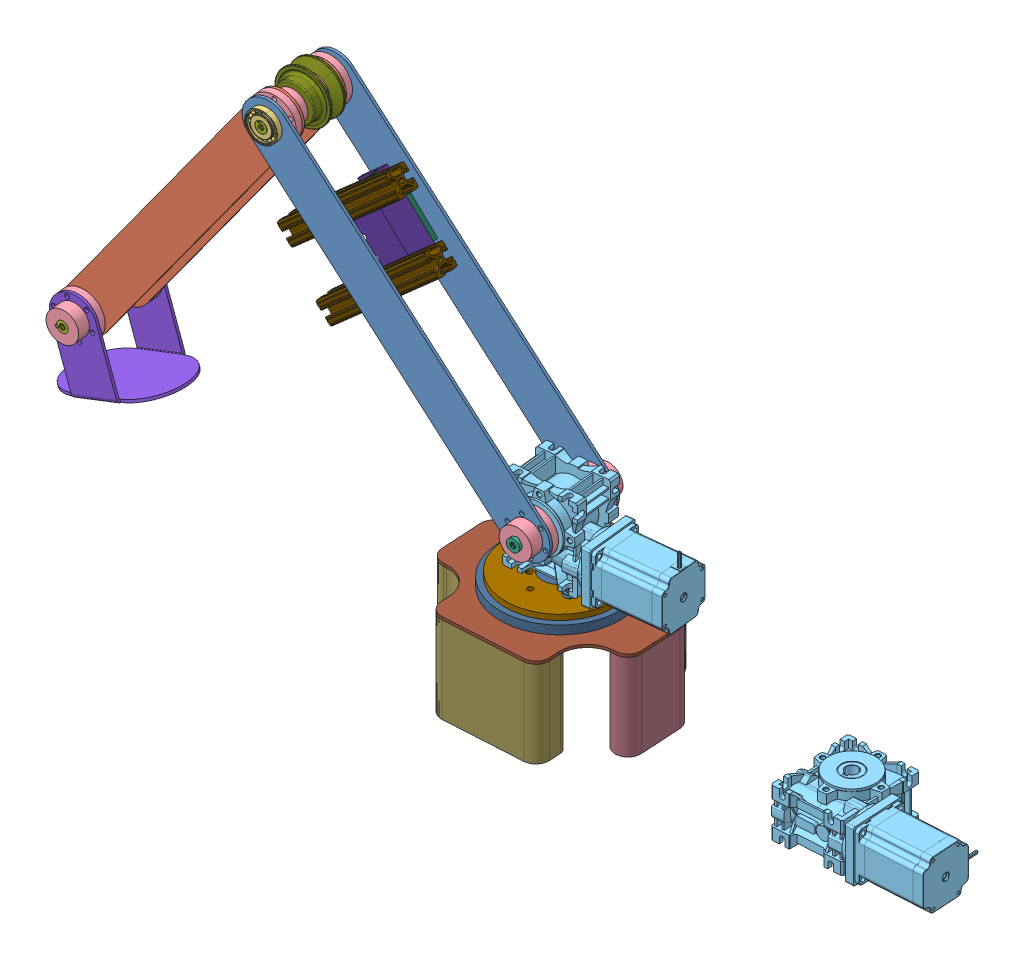
SolidWorks assembly Arm Assembly2, configuration Default. Lengths in mm.
Overall size (1007.94 520.17 219.18).
36 component instances, 19 part files, 85 mates.
Components (placement in the parent):
- Link 2-1: Link 2 [Default] at (47.0194 341.9058 298.1991) x (-0.680313 0.729219 0.073577) z (0.107525 0 0.994202) size (457.2 50.8 3.17)
- Link 3-1: Link 3 [Default] at (-260.6998 635.5723 404.1998) x (-0.575088 -0.815724 0.062197) z (0.107525 0 0.994202) size (406.4 50.8 3.17)
- Flanged Bearing-1: Flanged Bearing [Default] at (-450.225 330.8085 372.0961) x (0.994202 0 -0.107525) z (0.107525 0 0.994202) size (38.1 38.1 12.7)
- Keyed hub-1: Keyed hub [Default] at (37.3262 324.5251 380.8329) x (0.951664 -0.289383 -0.102924) z (-0.287705 -0.957214 0.031116) size (50.8 25.4 50.8)
- Link 2-2: Link 2 [Default] at (56.5945 341.9058 386.7328) x (-0.680313 0.729219 0.073577) z (0.107525 0 0.994202) size (457.2 50.8 3.17)
- Link 3-2: Link 3 [Default] at (-266.6726 635.5723 348.9744) x (-0.575088 -0.815724 0.062197) z (0.107525 0 0.994202) size (406.4 50.8 3.17)
- Flanged Bearing-2: Flanged Bearing [Default] at (-237.9498 620.8799 421.8585) x (-0.946563 0.30584 0.102372) z (0.107525 0 0.994202) size (38.1 38.1 12.7)
- Flanged Bearing-3: Flanged Bearing [Default] at (-444.6101 330.8085 424.0134) x (-0.918373 -0.383049 0.099324) z (-0.107525 0 -0.994202) size (38.1 38.1 12.7)
- Keyed hub-2: Keyed hub [Default] at (-246.9268 620.8799 338.8551) x (0.903538 0.417217 -0.097719) z (0.414798 -0.908807 -0.044861) size (50.8 25.4 50.8)
- Keyed hub-3: Keyed hub [Default] at (29.7995 324.5251 311.2388) x (-0.951664 0.289383 0.102924) z (-0.287705 -0.957214 0.031116) size (50.8 25.4 50.8)
- Keyed hub-4: Keyed hub [Default] at (-238.9057 620.8799 413.02) x (-0.903538 -0.417217 0.097719) z (0.414798 -0.908807 -0.044861) size (50.8 25.4 50.8)
- Flanged Bearing-4: Flanged Bearing [Default] at (-247.8827 620.8799 330.0166) x (0.915497 0.38995 -0.099013) z (-0.107525 0 -0.994202) size (38.1 38.1 12.7)
- Nema Stepper Motor-2: Nema Stepper Motor [Default] at (107.9306 305.5559 337.9928) x (0.994202 0 -0.107525) z (-0.107525 0 -0.994202) size (171.01 100.01 63.01)
- Nema Stepper Motor-3: Nema Stepper Motor [Default] at (426.1519 175.0272 335.1941) x (0.998228 0 -0.059501) z (0 -1 0) size (171.01 100.01 63.01)
- Keyed Drive Shaft-1: Keyed Drive Shaft [Default] at (22.6694 326.778 217.6376) x (0.951664 -0.289383 -0.102924) z (0.107525 0 0.994202) size (19.9 19.9 128.01)
- Keyed Shaft-1: Keyed Shaft [Default] at (-249.5571 620.8799 314.5343) x (0.903538 0.417217 -0.097719) z (0.107525 0 0.994202) size (12.7 12.5 104.14)
- Link 4-1: Link 4 [Default] at (-448.314 249.4662 399.083) x (0.107525 0 0.994202) z (-0.94726 -0.303649 0.102448) size (90.37 102.6 133.86)
- Keyed hub-5: Keyed hub [Default] at (-450.9818 330.8085 365.0987) x (0.301888 -0.952784 -0.03265) z (0.94726 0.303649 -0.102448) size (50.8 25.4 50.8)
- Keyed hub-6: Keyed hub [Default] at (-443.6542 330.8085 432.8518) x (-0.301888 0.952784 0.03265) z (0.94726 0.303649 -0.102448) size (50.8 25.4 50.8)
- Keyed Shaft-2: Keyed Shaft [Default] at (-439.8306 330.8085 468.2056) x (0.301888 -0.952784 -0.03265) z (-0.107525 0 -0.994202) size (12.7 12.5 104.14)
- Joint 2 Motor Plate-1: Joint 2 Motor Plate [Default] at (32.1724 257.1751 346.1862) x (0.994202 0 -0.107525) z (0.107525 0 0.994202) size (127 6.35 127)
- Bearing other part-1: Bearing other part [Default] at (32.1724 247.1751 346.1862) size (140 10 140)
- Top base plate-1: Top base plate [Default] at (33.5723 244.0001 346.2554) x (0.998228 0 -0.059501) z (0.059501 0 0.998228) size (222 3.17 194.94)
- arm base spacer large part-1: arm base spacer large part [Default] at (32.1724 142.4001 346.1862) x (-0.998228 0 0.059501) z (-0.059501 0 -0.998228) size (171.5 101.6 195.24)
- arm base spacer small part-1: arm base spacer small part [Default] at (130.8381 142.4001 364.6329) x (0.998228 0 -0.059501) z (0.059501 0 0.998228) size (30 101.6 78.26)
- 4 mm M6 spacer-1: 4 mm M6 spacer [94669A162] at (62.7675 265.5251 365.0056) x (-1 0 0) z (0 -1 0) size (13 13 4)
- 4 mm M6 spacer-2: 4 mm M6 spacer [94669A162] at (9.0806 260.6751 370.8119) x (1 0 0) z (0 -1 0) size (13 13 4)
- 4 mm M6 spacer-3: 4 mm M6 spacer [94669A162] at (58.0364 265.5251 321.2607) x (1 0 0) z (0 -1 0) size (13 13 4)
- 4 mm M6 spacer-4: 4 mm M6 spacer [94669A162] at (4.3495 260.6751 327.067) x (1 0 0) z (0 -1 0) size (13 13 4)
- 80 kg-1: 80 kg [Default] at (-156.7026 571.7069 383.4867) x (0.650213 -0.756491 -0.070322) z (0.752105 0.654004 -0.081341) size (82 48 30)
- 6204K122_Heavy Duty V-Belt Pulley.step-1: 6204K122_Heavy Duty V-Belt Pulley.step [Default] at (-243.7109 620.8799 368.59) x (0.584363 0.809027 -0.0632) z (0.107525 0 0.994202) size (59.69 59.69 31.75)
- servobracket_80kg-1: servobracket_80kg [Default] at (-150.7716 533.8316 383.6117) x (-0.650213 0.756491 0.070322) z (-0.752105 -0.654004 0.081341) size (87.12 31.24 59.67)
- 47065T553_T-Slotted Framing-1: 47065T553_T-Slotted Framing [47065T553] at (-124.2007 501.2106 393.5121) x (0.107525 0 0.994202) z (-0.752105 -0.654004 0.081341) size (25.4 25.4 152.4)
- 47065T553_T-Slotted Framing-2: 47065T553_T-Slotted Framing [47065T553] at (-165.4277 563.1313 397.9709) x (0.107525 0 0.994202) z (0.752105 0.654004 -0.081341) size (25.4 25.4 152.4)
- 91125A471_Female Threaded Round Standoff-2: 91125A471_Female Threaded Round Standoff [91125A471] at (-116.6227 514.5015 374.0424) x (0.994202 0 -0.107525) z (0.107525 0 0.994202) size (6.35 6.35 38.54)
- 91125A471_Female Threaded Round Standoff-3: 91125A471_Female Threaded Round Standoff [91125A471] at (-165.3886 571.2383 379.3165) x (0.978782 0.175445 -0.105857) z (0.107525 0 0.994202) size (6.35 6.35 38.54)
Mates (geometry in assembly coordinates):
- Concentric3: concentric aligned: cylinder of Keyed hub-1 through (38.1797 324.5251 388.7244) axis (0.107525 0 0.994202) radius 17.4625; cylinder of Link 2-2 through (38.1797 324.5251 388.7244) axis (0.107525 0 0.994202) radius 17.4625
- Coincident2: coincident anti-aligned: plane of Keyed hub-1 through (38.1797 324.5251 388.7244) normal (0.107525 0 0.994202); plane of Link 2-2 through (38.1797 324.5251 388.7244) normal (-0.107525 0 -0.994202)
- Concentric4: concentric aligned: cylinder of Keyed hub-1 through (58.2427 318.4244 386.5546) axis (0.107525 0 0.994202) radius 2.5527; cylinder of Link 2-2 through (58.5841 318.4244 389.7112) axis (0.107525 0 0.994202) radius 2.5527
- Concentric5: concentric anti-aligned: cylinder of Link 2-1 through (28.6046 324.5251 300.1907) axis (0.107525 0 0.994202) radius 17.4625; cylinder of Keyed hub-3 through (28.946 324.5251 303.3473) axis (-0.107525 0 -0.994202) radius 17.4625
- Coincident3: coincident anti-aligned: plane of Link 2-1 through (28.946 324.5251 303.3473) normal (0.107525 0 0.994202); plane of Keyed hub-3 through (28.946 324.5251 303.3473) normal (-0.107525 0 -0.994202)
- Concentric7: concentric anti-aligned: cylinder of Link 2-1 through (13.6617 310.0991 305.0003) axis (0.107525 0 0.994202) radius 2.5527; cylinder of Keyed hub-3 through (13.6617 310.0991 305.0003) axis (-0.107525 0 -0.994202) radius 2.5527
- Concentric8: concentric anti-aligned: cylinder of Keyed hub-1 through (37.3262 324.5251 380.8329) axis (0.107525 0 0.994202) radius 6.35; cylinder of Keyed hub-3 through (29.7995 324.5251 311.2388) axis (-0.107525 0 -0.994202) radius 6.35
- Coincident5: coincident aligned: plane of Keyed hub-1 through (35.8155 324.9845 380.9963) normal (0.951664 -0.289383 -0.102924); plane of Keyed hub-3 through (28.2887 324.9845 311.4022) normal (0.951664 -0.289383 -0.102924)
- Concentric9: concentric aligned: cylinder of Link 2-2 through (-238.2994 620.8799 418.6261) axis (0.107525 0 0.994202) radius 17.4625; cylinder of Flanged Bearing-2 through (-237.267 620.8799 428.1717) axis (0.107525 0 0.994202) radius 17.4625
- Concentric10: concentric anti-aligned: cylinder of Link 2-1 through (-247.8745 620.8799 330.0924) axis (0.107525 0 0.994202) radius 17.4625; cylinder of Flanged Bearing-4 through (-248.5655 620.8799 323.7034) axis (-0.107525 0 -0.994202) radius 17.4625
- Concentric11: concentric anti-aligned: cylinder of Link 3-1 through (-240.1006 620.8799 401.9719) axis (0.107525 0 0.994202) radius 17.4625; cylinder of Keyed hub-4 through (-239.7592 620.8799 405.1285) axis (-0.107525 0 -0.994202) radius 17.4625
- Coincident8: coincident anti-aligned: plane of Link 3-1 through (-239.7592 620.8799 405.1285) normal (0.107525 0 0.994202); plane of Keyed hub-4 through (-239.7592 620.8799 405.1285) normal (-0.107525 0 -0.994202)
- Concentric12: concentric anti-aligned: cylinder of Link 3-1 through (-256.8566 633.0746 406.9776) axis (0.107525 0 0.994202) radius 2.5527; cylinder of Keyed hub-4 through (-256.8566 633.0746 406.9776) axis (-0.107525 0 -0.994202) radius 2.5527
- Concentric13: concentric aligned: cylinder of Link 3-2 through (-246.0733 620.8799 346.7466) axis (0.107525 0 0.994202) radius 17.4625; cylinder of Keyed hub-2 through (-246.0733 620.8799 346.7466) axis (0.107525 0 0.994202) radius 17.4625
- Coincident9: coincident anti-aligned: plane of Link 3-2 through (-246.0733 620.8799 346.7466) normal (-0.107525 0 -0.994202); plane of Keyed hub-2 through (-246.0733 620.8799 346.7466) normal (0.107525 0 0.994202)
- Concentric14: concentric aligned: cylinder of Link 3-2 through (-262.8293 633.0746 351.7523) axis (0.107525 0 0.994202) radius 2.5527; cylinder of Keyed hub-2 through (-263.1707 633.0746 348.5957) axis (0.107525 0 0.994202) radius 2.5527
- Concentric15: concentric anti-aligned: cylinder of Keyed hub-2 through (-246.9268 620.8799 338.8551) axis (0.107525 0 0.994202) radius 6.35; cylinder of Keyed hub-4 through (-238.9057 620.8799 413.02) axis (-0.107525 0 -0.994202) radius 6.35
- Coincident10: coincident aligned: plane of Keyed hub-2 through (-245.4924 621.5422 338.7) normal (-0.903538 -0.417217 0.097719); plane of Keyed hub-4 through (-237.4713 621.5422 412.8649) normal (-0.903538 -0.417217 0.097719)
- Concentric16: concentric aligned: cylinder of Flanged Bearing-2 through (-237.267 620.8799 428.1717) axis (0.107525 0 0.994202) radius 6.35; cylinder of Keyed hub-2 through (-246.9268 620.8799 338.8551) axis (0.107525 0 0.994202) radius 6.35
- Concentric17: concentric aligned: cylinder of Flanged Bearing-1 through (-449.5422 330.8085 378.4093) axis (0.107525 0 0.994202) radius 17.4625; cylinder of Link 3-2 through (-450.5746 330.8085 368.8638) axis (0.107525 0 0.994202) radius 17.4625
- Coincident13: coincident anti-aligned: plane of Flanged Bearing-1 through (-450.5746 348.271 368.8638) normal (0.107525 0 0.994202); plane of Link 3-2 through (-246.0733 620.8799 346.7466) normal (-0.107525 0 -0.994202)
- Concentric18: concentric anti-aligned: cylinder of Link 3-1 through (-444.6019 330.8085 424.0891) axis (0.107525 0 0.994202) radius 17.4625; cylinder of Flanged Bearing-3 through (-445.2929 330.8085 417.7002) axis (-0.107525 0 -0.994202) radius 17.4625
- Coincident14: coincident anti-aligned: plane of Link 3-1 through (-239.7592 620.8799 405.1285) normal (0.107525 0 0.994202); plane of Flanged Bearing-3 through (-450.9107 346.9391 427.9649) normal (-0.107525 0 -0.994202)
- Concentric21: concentric anti-aligned: cylinder of Keyed hub-1 through (37.3262 324.5251 380.8329) axis (0.107525 0 0.994202) radius 6.35; cylinder of Keyed Drive Shaft-1 through (40.4444 324.5251 409.6648) axis (-0.107525 0 -0.994202) radius 7
- Parallel1: parallel anti-aligned: plane of Keyed hub-1 through (35.8155 324.9845 380.9963) normal (0.951664 -0.289383 -0.102924); plane of Keyed Drive Shaft-1 through (32.7085 330.3218 346.1282) normal (-0.951664 0.289383 0.102924)
- Coincident18: coincident anti-aligned: plane of Keyed hub-3 through (29.7995 324.5251 311.2388) normal (0.107525 0 0.994202); plane of Keyed Drive Shaft-1 through (30.5832 331.2793 311.154) normal (-0.107525 0 -0.994202)
- Coincident19: coincident anti-aligned: plane of Keyed hub-1 through (37.3262 324.5251 380.8329) normal (-0.107525 0 -0.994202); plane of Keyed Drive Shaft-1 through (38.1099 331.2793 380.7482) normal (0.107525 0 0.994202)
- Concentric22: concentric anti-aligned: cylinder of Keyed hub-2 through (-246.9268 620.8799 338.8551) axis (0.107525 0 0.994202) radius 6.35; cylinder of Keyed Shaft-1 through (-237.267 620.8799 428.1717) axis (-0.107525 0 -0.994202) radius 6.35
- Coincident20: coincident aligned: plane of Keyed hub-2 through (-245.4924 621.5422 338.7) normal (-0.903538 -0.417217 0.097719); plane of Keyed Shaft-1 through (-237.8029 625.8589 428.2296) normal (-0.903538 -0.417217 0.097719)
- Coincident22: coincident anti-aligned: plane of Link 2-1 through (28.946 324.5251 303.3473) normal (0.107525 0 0.994202); plane of Flanged Bearing-4 through (-240.7631 604.7998 332.5168) normal (-0.107525 0 -0.994202)
- Distance1: distance = 2.54 mm anti-aligned: plane of Flanged Bearing-4 through (-242.7391 610.2846 335.8474) normal (0.107525 0 0.994202); plane of Keyed hub-2 through (-246.9268 620.8799 338.8551) normal (-0.107525 0 -0.994202)
- Coincident24: coincident anti-aligned: plane of Link 2-2 through (38.1797 324.5251 388.7244) normal (-0.107525 0 -0.994202); plane of Flanged Bearing-2 through (-243.6092 604.2542 419.2004) normal (0.107525 0 0.994202)
- Distance2: distance = 2.54 mm anti-aligned: plane of Keyed hub-4 through (-238.9057 620.8799 413.02) normal (0.107525 0 0.994202); plane of Flanged Bearing-2 through (-242.1312 609.925 415.9237) normal (-0.107525 0 -0.994202)
- Coincident26: coincident aligned: plane of Flanged Bearing-2 through (-239.1979 614.8342 428.3805) normal (0.107525 0 0.994202); plane of Keyed Shaft-1 through (-237.267 620.8799 428.1717) normal (0.107525 0 0.994202)
- Concentric23: concentric anti-aligned: cylinder of Link 4-1 through (-442.4593 330.8085 443.8999) axis (-0.107525 0 -0.994202) radius 17.4625; cylinder of Keyed hub-6 through (-442.8007 330.8085 440.7433) axis (0.107525 0 0.994202) radius 17.4625
- Concentric24: concentric anti-aligned: cylinder of Link 4-1 through (-463.2776 335.3079 442.9579) axis (-0.107525 0 -0.994202) radius 2.5527; cylinder of Keyed hub-6 through (-463.2776 335.3079 442.9579) axis (0.107525 0 0.994202) radius 2.5527
- Coincident27: coincident anti-aligned: plane of Link 4-1 through (-431.415 210.3886 439.5119) normal (-0.107525 0 -0.994202); plane of Keyed hub-6 through (-442.8007 330.8085 440.7433) normal (0.107525 0 0.994202)
- Concentric25: concentric anti-aligned: cylinder of Link 4-1 through (-452.1767 330.8085 354.0506) axis (0.107525 0 0.994202) radius 17.4625; cylinder of Keyed hub-5 through (-451.8353 330.8085 357.2072) axis (-0.107525 0 -0.994202) radius 17.4625
- Concentric26: concentric anti-aligned: cylinder of Link 4-1 through (-472.3121 335.3079 359.4218) axis (0.107525 0 0.994202) radius 2.5527; cylinder of Keyed hub-5 through (-472.3121 335.3079 359.4218) axis (-0.107525 0 -0.994202) radius 2.5527
- Concentric27: concentric anti-aligned: cylinder of Keyed hub-5 through (-450.9818 330.8085 365.0987) axis (-0.107525 0 -0.994202) radius 6.35; cylinder of Keyed Shaft-2 through (-452.1207 330.8085 354.5683) axis (0.107525 0 0.994202) radius 6.35
- Coincident31: coincident aligned: plane of Keyed hub-5 through (-451.4611 332.3211 365.1505) normal (0.301888 -0.952784 -0.03265); plane of Keyed Shaft-2 through (-457.0992 330.8788 355.1068) normal (0.301888 -0.952784 -0.03265)
- Coincident32: coincident aligned: plane of Keyed hub-6 through (-440.9231 330.8085 458.1046) normal (0.107525 0 0.994202); plane of Keyed Shaft-2 through (-440.9231 330.8085 458.1046) normal (0.107525 0 0.994202)
- Coincident34: coincident anti-aligned: plane of Link 4-1 through (-440.4496 210.3886 355.9758) normal (0.107525 0 0.994202); plane of Keyed hub-5 through (-451.8353 330.8085 357.2072) normal (-0.107525 0 -0.994202)
- Coincident36: coincident aligned: plane of Keyed hub-6 through (-443.1749 329.296 432.8) normal (-0.301888 0.952784 0.03265); plane of Keyed Shaft-2 through (-456.1407 327.8537 355.0031) normal (-0.301888 0.952784 0.03265)
- Concentric28: concentric anti-aligned: cone of Flanged Bearing-3 through (-443.9993 330.8085 429.6608) axis (-0.107525 0 -0.994202); cylinder of Keyed Shaft-2 through (-452.1207 330.8085 354.5683) axis (0.107525 0 0.994202) radius 6.35
- Distance3: distance = 2.54 mm anti-aligned: plane of Flanged Bearing-3 through (-448.3092 341.4371 430.8004) normal (0.107525 0 0.994202); plane of Keyed hub-6 through (-443.6542 330.8085 432.8518) normal (-0.107525 0 -0.994202)
- Coincident37: coincident anti-aligned: plane of Bearing maybe-1 through (32.1724 257.1751 346.1862) normal (0 -1 0); plane of Bearing other part-1 through (32.1724 257.1751 346.1862) normal (0 1 0)
- Concentric29: concentric aligned: cylinder of Bearing maybe-1 through (32.1724 263.5251 346.1862) axis (0 -1 0) radius 63.5; cylinder of Bearing other part-1 through (32.1724 257.1751 346.1862) axis (0 -1 0) radius 70
- Coincident38: coincident anti-aligned: plane of Top base plate-1 through (74.0847 244.0001 261.2257) normal (0 -1 0); plane of arm base spacer small part-1 through (130.8381 244.0001 364.6329) normal (0 1 0)
- Coincident40: coincident anti-aligned: plane of Top base plate-1 through (74.0847 244.0001 261.2257) normal (0 -1 0); plane of arm base spacer large part-1 through (32.1724 244.0001 346.1862) normal (0 1 0)
- Coincident45: coincident anti-aligned: plane of Bearing other part-1 through (32.1724 247.1751 346.1862) normal (0 -1 0); plane of Top base plate-1 through (74.0847 247.1751 261.2257) normal (0 1 0)
- Concentric32: concentric aligned: cylinder of Bearing other part-1 through (32.1724 257.1751 346.1862) axis (0 -1 0) radius 70; circle of arm base spacer large part-1
- Coincident50: coincident anti-aligned: plane of Bearing maybe-1 through (32.1724 263.5251 346.1862) normal (0 1 0); plane of 4 mm M6 spacer-3 through (58.0364 263.5251 321.2607) normal (0 -1 0)
- Coincident55: coincident anti-aligned: plane of Nema Stepper Motor-2 through (107.9306 305.5559 337.9928) normal (-0.107525 0 -0.994202); plane of Bearing maybe-1 through (32.1724 257.1751 346.1862) normal (0.107525 0 0.994202)
- Distance5: distance = 76.2 mm aligned: plane of Nema Stepper Motor-2 through (107.9306 305.5559 337.9928) normal (0.994202 0 -0.107525); plane of Bearing maybe-1 through (32.1724 257.1751 346.1862) normal (0.994202 0 -0.107525)
- Coincident57: coincident aligned: plane of Top base plate-1 through (-6.0476 247.1751 446.2586) normal (0.059501 0 0.998228); plane of arm base spacer large part-1 through (84.7912 244.0001 440.844) normal (0.059501 0 0.998228)
- Coincident58: coincident aligned: plane of Top base plate-1 through (-75.7951 247.1751 376.9496) normal (-0.998228 0 0.059501); plane of arm base spacer large part-1 through (-75.8042 244.0001 376.7975) normal (-0.998228 0 0.059501)
- Concentric37: concentric aligned: cylinder of Top base plate-1 through (130.8381 247.1751 364.6329) axis (0 -1 0) radius 15; cylinder of arm base spacer small part-1 through (130.8381 244.0001 364.6329) axis (0 -1 0) radius 15
- Coincident59: coincident aligned: plane of Top base plate-1 through (145.8116 247.1751 363.7404) normal (0.998228 0 -0.059501); plane of arm base spacer small part-1 through (145.8116 244.0001 363.7404) normal (0.998228 0 -0.059501)
- Parallel2: parallel aligned: plane of Nema Stepper Motor-3 through (350.3499 203.0272 320.7095) normal (0 1 0); plane of Top base plate-1 through (74.0847 247.1751 261.2257) normal (0 1 0)
- Parallel3: parallel anti-aligned: plane of Nema Stepper Motor-3 through (312.2058 175.0272 353.0364) normal (-0.998228 0 0.059501); plane of arm base spacer small part-1 through (145.8116 244.0001 363.7404) normal (0.998228 0 -0.059501)
- Coincident61: coincident anti-aligned: plane of Nema Stepper Motor-2 through (76.3373 267.5251 369.573) normal (0 -1 0); plane of 4 mm M6 spacer-1 through (62.7675 267.5251 365.0056) normal (0 1 0)
- Concentric39: concentric aligned: cylinder of Nema Stepper Motor-2 through (62.7675 364.5251 365.0056) axis (0 -1 0) radius 3.25; cylinder of 4 mm M6 spacer-1 through (62.7675 267.5251 365.0056) axis (0 -1 0) radius 3.15
- Coincident62: coincident anti-aligned: plane of Bearing maybe-1 through (32.1724 263.5251 346.1862) normal (0 1 0); plane of 4 mm M6 spacer-1 through (62.7675 263.5251 365.0056) normal (0 -1 0)
- Concentric40: concentric aligned: cylinder of Nema Stepper Motor-2 through (58.0364 364.5251 321.2607) axis (0 -1 0) radius 3.25; cylinder of 4 mm M6 spacer-3 through (58.0364 267.5251 321.2607) axis (0 -1 0) radius 3.15
- Concentric41: concentric aligned: cylinder of Nema Stepper Motor-2 through (4.3495 364.5251 327.067) axis (0 -1 0) radius 3.25; cylinder of 4 mm M6 spacer-4 through (4.3495 262.6751 327.067) axis (0 -1 0) radius 3.15
- Concentric42: concentric aligned: cylinder of Nema Stepper Motor-2 through (9.0806 364.5251 370.8119) axis (0 -1 0) radius 3.25; cylinder of 4 mm M6 spacer-2 through (9.0806 262.6751 370.8119) axis (0 -1 0) radius 3.15
- Concentric43: concentric aligned: cylinder of Keyed hub-1 through (38.1797 324.5251 388.7244) axis (0.107525 0 0.994202) radius 17.4625; cylinder of Nema Stepper Motor-2 through (23.5926 324.5251 253.848) axis (0.107525 0 0.994202) radius 7
- Coincident65: coincident anti-aligned: plane of Nema Stepper Motor-2 through (36.9455 324.5251 377.3537) normal (0.107525 0 0.994202); plane of Keyed Drive Shaft-1 through (36.9499 324.5251 377.3532) normal (-0.107525 0 -0.994202)
- Concentric44: concentric aligned: cylinder of 80 kg-1 through (-128.8622 503.3834 380.4757) axis (-0.107525 0 -0.994202) radius 3; cylinder of servobracket_80kg-1 through (-128.7803 503.3834 381.2333) axis (-0.107525 0 -0.994202) radius 3
- Coincident77: coincident anti-aligned: circle of 80 kg-1; cylinder of servobracket_80kg-1 through (-115.9945 514.5015 379.8505) axis (-0.107525 0 -0.994202) radius 3
- Concentric45: concentric aligned: cylinder of 80 kg-1 through (-177.6282 560.1202 385.7499) axis (-0.107525 0 -0.994202) radius 3; cylinder of servobracket_80kg-1 through (-177.5462 560.1202 386.5074) axis (-0.107525 0 -0.994202) radius 3
- Concentric46: concentric aligned: cylinder of 80 kg-1 through (-164.8424 571.2383 384.367) axis (-0.107525 0 -0.994202) radius 3; cylinder of servobracket_80kg-1 through (-164.7604 571.2383 385.1246) axis (-0.107525 0 -0.994202) radius 3
- Concentric47: concentric anti-aligned: cylinder of Keyed Shaft-1 through (-237.267 620.8799 428.1717) axis (-0.107525 0 -0.994202) radius 6.35; cylinder of 6204K122_Heavy Duty V-Belt Pulley.step-1 through (-242.0039 620.8799 384.373) axis (0.107525 0 0.994202) radius 7.9375
- Coincident80: coincident anti-aligned: plane of 80 kg-1 through (-156.7026 571.7069 383.4867) normal (0.107525 0 0.994202); plane of servobracket_80kg-1 through (-150.8535 533.8316 382.8541) normal (-0.107525 0 -0.994202)
- Coincident81: coincident anti-aligned: plane of Link 2-2 through (38.1797 324.5251 388.7244) normal (-0.107525 0 -0.994202); plane of 47065T553_T-Slotted Framing-1 through (-177.4209 448.2055 412.042) normal (0.107525 0 0.994202)
- Coincident82: coincident anti-aligned: plane of servobracket_80kg-1 through (-150.7716 533.8316 383.6117) normal (0.107525 0 0.994202); plane of 47065T553_T-Slotted Framing-1 through (-185.6013 454.5454 387.3786) normal (-0.107525 0 -0.994202)
- Parallel5: parallel anti-aligned: line of servobracket_80kg-1 through (-103.3442 517.4898 378.4824) axis (-0.752105 -0.654004 0.081341); line of 47065T553_T-Slotted Framing-1 through (-176.5021 443.959 386.3945) axis (0.752105 0.654004 -0.081341)
- Coincident85: coincident anti-aligned: plane of Link 2-2 through (38.1797 324.5251 388.7244) normal (-0.107525 0 -0.994202); plane of 47065T553_T-Slotted Framing-2 through (-109.4764 616.1364 404.6937) normal (0.107525 0 0.994202)
- Coincident86: coincident anti-aligned: plane of servobracket_80kg-1 through (-150.7716 533.8316 383.6117) normal (0.107525 0 0.994202); plane of 47065T553_T-Slotted Framing-2 through (-106.7583 609.7964 378.8516) normal (-0.107525 0 -0.994202)
- Parallel6: parallel anti-aligned: line of servobracket_80kg-1 through (-198.1989 550.1733 388.7411) axis (0.752105 0.654004 -0.081341); line of 47065T553_T-Slotted Framing-2 through (-115.8574 620.3828 379.8357) axis (-0.752105 -0.654004 0.081341)
- Concentric51: concentric anti-aligned: cylinder of servobracket_80kg-1 through (-115.9945 514.5015 379.8505) axis (-0.107525 0 -0.994202) radius 3; cone of 91125A471_Female Threaded Round Standoff-2 through (-118.671 514.5015 355.1028) axis (0.107525 0 0.994202)
- Coincident87: coincident anti-aligned: plane of servobracket_80kg-1 through (-150.8535 533.8316 382.8541) normal (-0.107525 0 -0.994202); plane of 91125A471_Female Threaded Round Standoff-2 through (-116.0764 514.5015 379.0929) normal (0.107525 0 0.994202)
- Concentric53: concentric anti-aligned: cylinder of servobracket_80kg-1 through (-164.7604 571.2383 385.1246) axis (-0.107525 0 -0.994202) radius 3; cone of 91125A471_Female Threaded Round Standoff-3 through (-167.437 571.2383 360.3769) axis (0.107525 0 0.994202)
- Coincident89: coincident anti-aligned: plane of servobracket_80kg-1 through (-150.8535 533.8316 382.8541) normal (-0.107525 0 -0.994202); plane of 91125A471_Female Threaded Round Standoff-3 through (-164.8424 571.2383 384.367) normal (0.107525 0 0.994202)
